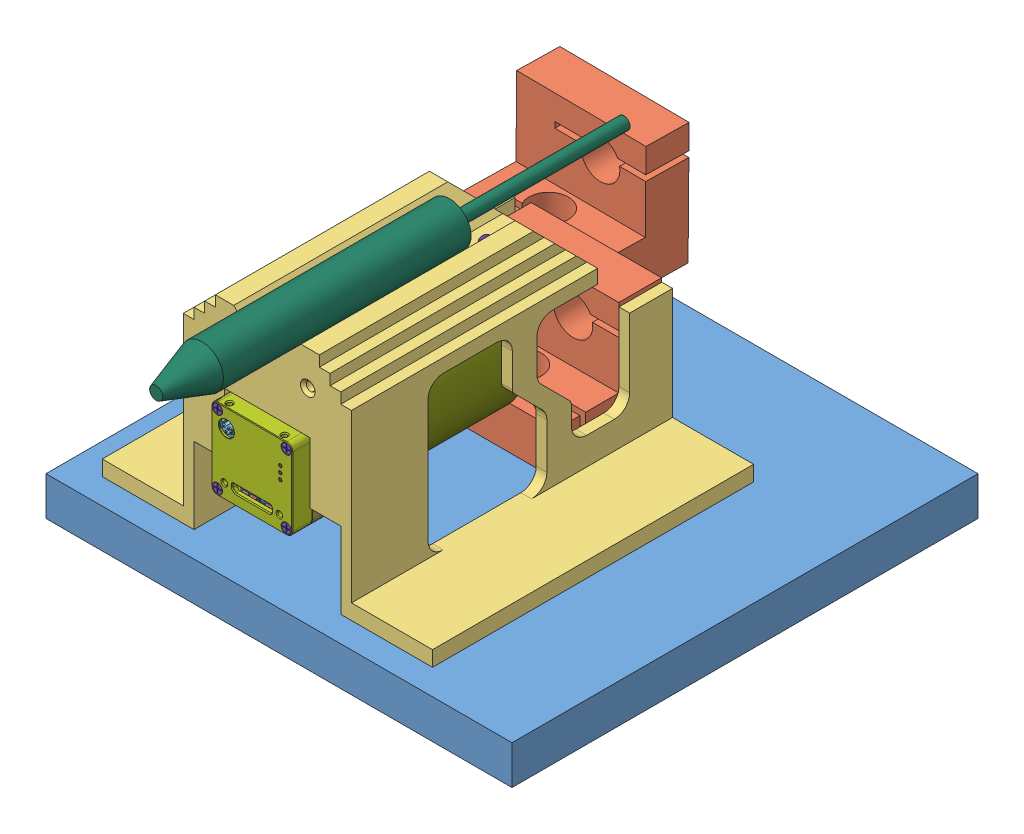
SolidWorks assembly system, configuration Default. Lengths in mm.
Overall size (152.4 91.45 195.72).
56 component instances, 36 part files, 3 mates.
Components (placement in the parent):
- plate-2: plate [Default] x (1 0 0) z (0 -1 0) size (152.4 152.4 12.7)
- galvo_block-1: galvo_block [Default] at (-75.8464 11.6774 -91.2725) x (-0.000076 -0.999962 0.008726) z (0.999962 0 0.008727) size (39.65 34.73 42.65)
- cam_assem-1: cam_assem [Default] at (-12.1559 45 42.8466) size (108 78.75 153)
  - cam_holder-1: cam_holder [Default] at origin size (108 78.73 105)
  - STP-MQ-(MQ022xG-CM)-ASSM-1: STP-MQ-(MQ022xG-CM)-ASSM [Default] at (0 -13.2 7.5) x (-1 0 0) z (0 0 -1) size (26.4 26.4 30.19)
    - STP-MQ-(MQ022xG-CM)-ASSM.stp-1: STP-MQ-(MQ022xG-CM)-ASSM.stp [Default] at origin size (26.4 26.4 30.19)
      - SUBASSM-MQ-FRONT.stp-1: SUBASSM-MQ-FRONT.stp [Default] x (0 -1 0) z (0 0 1) size (26.4 26.4 14.6)
        - MECH-MQ-FRONT.stp-1: MECH-MQ-FRONT.stp [Default] at (0 0 7.5) x (1 0 0) z (0 0 -1) size (26.4 26.4 7.5)
        - MECH-MQ-CS-C.stp-1: MECH-MQ-CS-C.stp [Default] at (0 0 0.5) x (1 0 0) z (0 0 -1) size (26.4 26.4 5.5)
        - SROB-M2x14-CUST.stp-1: SROB-M2x14-CUST.stp [Default] at (-11.25 11.25 -7.1) size (3 3 14.55)
        - SROB-M2x14-CUST.stp-2: SROB-M2x14-CUST.stp [Default] at (11.25 -11.25 -7.1) size (3 3 14.55)
        - SROB-M2x14-CUST.stp-3: SROB-M2x14-CUST.stp [Default] at (11.25 11.25 -7.1) size (3 3 14.55)
        - SROB-M2x14-CUST.stp-4: SROB-M2x14-CUST.stp [Default] at (-11.25 -11.25 -7.1) size (3 3 14.55)
      - SUBASSM-MQ-REAR.stp-1: SUBASSM-MQ-REAR.stp [Default] at (0 0 -22.584) x (-1 0 0) z (0 0 1) size (26.4 26.4 10.6)
        - MECH-MQ-REAR.stp-1: MECH-MQ-REAR.stp [Default] at (0 0 6.5) x (-1 0 0) z (0 0 -1) size (26.4 26.4 6.5)
        - SROB-M2x10-CUST .stp-1: SROB-M2x10-CUST .stp [Default] at (-11.25 11.25 10.6) x (1 0 0) z (0 0 -1) size (3 3 10.55)
        - SROB-M2x10-CUST .stp-2: SROB-M2x10-CUST .stp [Default] at (11.25 11.25 10.6) x (1 0 0) z (0 0 -1) size (3 3 10.55)
        - SROB-M2x10-CUST .stp-3: SROB-M2x10-CUST .stp [Default] at (11.25 -11.25 10.6) x (1 0 0) z (0 0 -1) size (3 3 10.55)
        - SROB-M2x10-CUST .stp-4: SROB-M2x10-CUST .stp [Default] at (-11.25 -11.25 10.6) x (1 0 0) z (0 0 -1) size (3 3 10.55)
        - MECH-MQ-THERMAL-PAD.stp-1: MECH-MQ-THERMAL-PAD.stp [Default] at (-10.5 5.45 4.8) x (0.961741 -0.273959 0) z (0 0 -1) size (20.28 8 0.5)
        - MECH-EMI-GSKT-1.3X2.3X11.stp-1: MECH-EMI-GSKT-1.3X2.3X11.stp [Default] at (0 9.9495 3.45) size (11 1.2 3)
        - MECH-EMI-GSKT-1.3X2.3X11.stp-2: MECH-EMI-GSKT-1.3X2.3X11.stp [Default] at (0 7.0505 3.45) size (11 1.2 3)
        - MECH-LIGHTPIPE-1.63X4.14.stp-1: MECH-LIGHTPIPE-1.63X4.14.stp [Default] at (9.3 -3.5 4.1492) x (-1 0 0) z (0 -1 0) size (1.63 4.14 1.63)
        - MECH-LIGHTPIPE-1.63X4.14.stp-2: MECH-LIGHTPIPE-1.63X4.14.stp [Default] at (9.3 -1.5 4.1492) x (-1 0 0) z (0 -1 0) size (1.63 4.14 1.63)
        - MECH-LIGHTPIPE-1.63X4.14.stp-3: MECH-LIGHTPIPE-1.63X4.14.stp [Default] at (9.3 -5.5 4.1492) x (-1 0 0) z (0 -1 0) size (1.63 4.14 1.63)
      - SUBASSM-MQ-MID-022-CM.stp-1: SUBASSM-MQ-MID-022-CM.stp [Default] at (0 0 -4.5) x (-1 0 0) z (0 0 -1) size (26.4 26.4 11.68)
        - MECH-MQ-MID-022-CM-REV2.stp-1: MECH-MQ-MID-022-CM-REV2.stp [Default] at origin size (26.4 26.4 11.59)
        - MECH-O-RING-22X1-VI370.stp-1: MECH-O-RING-22X1-VI370.stp [Default] at (0 0 1.3) x (1 0 0) z (0 1 0) size (24 1 24)
        - FLT-BK7-AR2X-D25.stp-1: FLT-BK7-AR2X-D25.stp [Default] at (0 0 -0.1) size (25 25 1.1)
        - MECH-MX022xG-CM-GSKT.stp-1: MECH-MX022xG-CM-GSKT.stp [Default] at (0 0 3.364) x (0 -1 0) z (0 0 1) size (12.2 17.4 1.27)
      - MQ022xG-CM-PCA-LW_MODEL.stp-1: MQ022xG-CM-PCA-LW_MODEL.stp [Default] at (0 0 -16.486) x (-1 0 0) z (0 0 -1) size (25.43 25.43 13.85)
        - CMV2000.stp-1: CMV2000.stp [Default] at (-0.0259 -0.5261 -1.002) x (-1 0 0) z (0 0 -1) size (18.65 13.5 6.65)
          - ANDON-96UPGA-Socket.stp-1: ANDON-96UPGA-Socket.stp [Default] at origin size (15.9 10.8 3.23)
          - CMV2000_Package.stp-1: CMV2000_Package.stp [Default] at (0 0 3.29) x (-1 0 0) z (0 0 1) size (18.65 13.5 5.45)
          - CMV2000_Glass.stp-1: CMV2000_Glass.stp [Default] at (0 0 6.1) size (18.06 12.95 0.55)
        - MQ022xG-CM-PCA-LW_MODEL-0.stp-1: MQ022xG-CM-PCA-LW_MODEL-0.stp [Default] at origin size (0.25 1.57 4.1)
        - MQ022xG-CM-PCA-LW_MODEL-1.stp-1: MQ022xG-CM-PCA-LW_MODEL-1.stp [Default] at origin size (12.85 2.05 3.8)
        - MQ022xG-CM-PCA-LW_MODEL-2.stp-1: MQ022xG-CM-PCA-LW_MODEL-2.stp [Default] at origin size (25.43 25.43 1)
        - MQ022xG-CM-PCA-LW_MODEL-3.stp-1: MQ022xG-CM-PCA-LW_MODEL-3.stp [Default] at origin size (0.25 1.57 4.1)
        - MQ022xG-CM-PCA-LW_MODEL-4.stp-1: MQ022xG-CM-PCA-LW_MODEL-4.stp [Default] at origin size (5 5 8.1)
        - MQ022xG-CM-PCA-LW_MODEL-5.stp-1: MQ022xG-CM-PCA-LW_MODEL-5.stp [Default] at origin size (0.25 1.57 4.1)
        - MQ022xG-CM-PCA-LW_MODEL-6.stp-1: MQ022xG-CM-PCA-LW_MODEL-6.stp [Default] at origin size (0.25 1.57 4.1)
        - MQ022xG-CM-PCA-LW_MODEL-7.stp-1: MQ022xG-CM-PCA-LW_MODEL-7.stp [Default] at origin size (0.25 1.57 4.1)
        - MQ022xG-CM-PCA-LW_MODEL-8.stp-1: MQ022xG-CM-PCA-LW_MODEL-8.stp [Default] at origin size (0.25 1.57 4.1)
        - MQ022xG-CM-PCA-LW_MODEL-9.stp-1: MQ022xG-CM-PCA-LW_MODEL-9.stp [Default] at origin size (0.25 1.57 4.1)
        - MQ022xG-CM-PCA-LW_MODEL-10.stp-1: MQ022xG-CM-PCA-LW_MODEL-10.stp [Default] at origin size (0.25 1.57 4.1)
        - MQ022xG-CM-PCA-LW_MODEL-11.stp-1: MQ022xG-CM-PCA-LW_MODEL-11.stp [Default] at origin size (0.25 1.57 4.1)
        - MQ022xG-CM-PCA-LW_MODEL-12.stp-1: MQ022xG-CM-PCA-LW_MODEL-12.stp [Default] at origin size (13.8 3 5.6)
        - MQ022xG-CM-PCA-LW_MODEL-13.stp-1: MQ022xG-CM-PCA-LW_MODEL-13.stp [Default] at origin size (0.25 1.57 4.1)
  - laser-1: laser [Default] at (0 23.8995 -34.6198) x (0.771778 -0.635892 0) z (0 0 1) size (14 14 153)
  - lens-1: lens [Default] at (0 -13.2 -42) x (0 1 0) z (0 0 1) size (33.5 33.5 46.7)
  - 1598K25_Hardened Bearing-Quality 440C Stainless Steel Ball-1: 1598K25_Hardened Bearing-Quality 440C Stainless Steel Ball [1598K25] at (-7.5476 19.1804 20) x (0.280446 0.805937 0.52136) z (-0.678439 -0.217803 0.701628) size (4 4 4)
  - 92695A729_Alloy Steel Cone-Point Set Screws-1: 92695A729_Alloy Steel Cone-Point Set Screws [92695A729] at (-8.4914 18.3374 24.4029) x (0.913011 -0.407935 0) z (0 0 1) size (4.05 3.54 3.43)
  - 1598K25_Hardened Bearing-Quality 440C Stainless Steel Ball-2: 1598K25_Hardened Bearing-Quality 440C Stainless Steel Ball [1598K25] at (-6.7175 19.0104 -40) x (0.756378 0.1991 0.623098) z (-0.446406 -0.539153 0.714168) size (4 4 4)
  - 1598K25_Hardened Bearing-Quality 440C Stainless Steel Ball-4: 1598K25_Hardened Bearing-Quality 440C Stainless Steel Ball [1598K25] at (6.7175 19.0104 -40) x (0.295652 0.723786 0.623477) z (-0.259043 -0.567459 0.781593) size (4 4 4)
  - galvo_block-1: galvo_block [Default] at (-18.725 -27.865 -80) x (0 -1 0) z (1 0 0) size (39.65 34.73 42.65)
Mates (geometry in assembly coordinates):
- Coincident12: coincident: point of plate-2
- Coincident11: coincident anti-aligned: plane of plate-2 through (0 0 0) normal (0 -1 0)
- Coincident13: coincident anti-aligned: plane of plate-2 through (0 0 0) normal (0 1 0); plane of cam_assem-1/cam_holder-1 through (-36.1559 0 67.8466) normal (0 -1 0)
